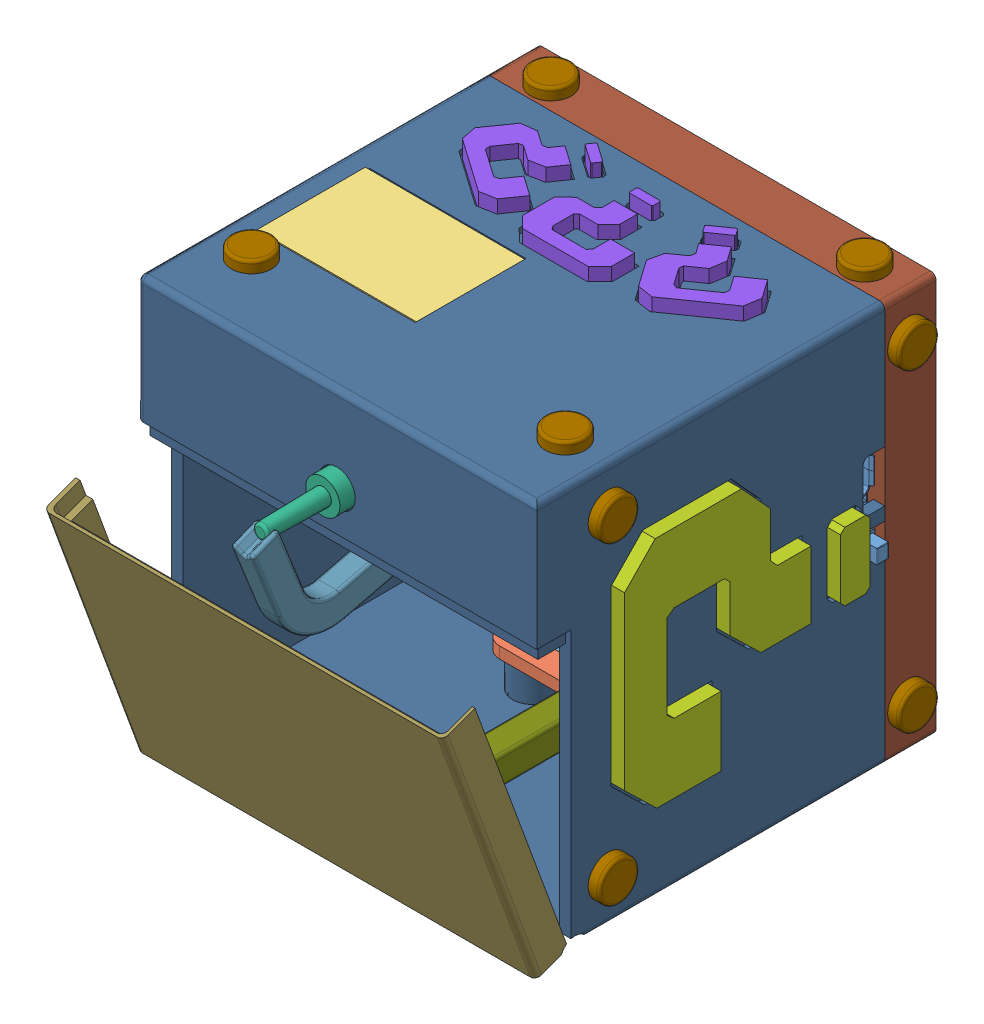
SolidWorks assembly 舔狗马里奥, configuration 默认. Lengths in mm.
Overall size (74.78 77.95 86.83).
34 component instances, 16 part files, 58 mates.
Components (placement in the parent):
- PCBA-1: PCBA [默认] at origin size (51.47 38.47 13.02)
- MP3模块-1: MP3模块 [默认] at (25.9874 -44.631 -27.0444) x (1 0 0) z (0 -1 0) size (40 32.5 9.5)
- OLED模块-1: OLED模块 [默认] at (-29.2626 11.569 29.8364) x (-1 0 0) z (0 1 0) size (28.5 28 22)
- 电池-1: 电池 [默认] at (-22.5126 -20.181 -82.6) x (0 0 -1) z (1 0 0) size (35.65 51.27 10)
- MG90S舵机-1: MG90S舵机 [默认] at (45.3874 0.569 27.75) x (0 0 1) z (0 -1 0) size (32.5 30.4 12.5)
- MG90S舵机-2: MG90S舵机 [默认] at (35.9874 -6.431 26.15) x (0 0 1) z (1 0 0) size (32.5 30.4 12.5)
- 开关-1: 开关 [默认] at (12.9874 0.569 47.9) x (-1 0 0) z (0 1 0) size (13 33 10)
- 马里奥问号-1: 马里奥问号 [默认] at (-21.0126 -25.4863 24.1423) x (0 1 0) z (0 0 1) size (41.06 3 43.04)
- 马里奥问号-2: 马里奥问号 [默认] at (18.3797 -53.431 24.146) x (-1 0 0) z (0 0 1) size (41.06 3 43.04)
- 马里奥问号-3: 马里奥问号 [默认] at (46.9874 -13.3946 24.3671) x (0 -1 0) z (0 0 1) size (41.06 3 43.04)
- 马里奥小问号-1: 马里奥小问号 [默认] at (-113.1118 14.569 -50.476) size (51.04 3 19.45)
- 马里奥键帽-1: 马里奥键帽 [默认] at (-21.0126 8.069 49.9) x (0 0.999538 0.03038) z (0 -0.03038 0.999538) size (7 3 7)
- 马里奥键帽-5: 马里奥键帽 [默认] at (-14.5126 -53.431 49.9) x (-0.990543 0 0.137199) z (0.137199 0 0.990543) size (7 3 7)
- 马里奥键帽-9: 马里奥键帽 [默认] at (46.9874 -46.931 49.9) x (0 -0.948117 -0.317921) z (0 -0.317921 0.948117) size (7 3 7)
- 马里奥键帽-13: 马里奥键帽 [默认] at (40.4874 14.569 49.9) x (0.738275 0 -0.6745) z (0.6745 0 0.738275) size (7 3 7)
- 马里奥盒子主体-1: 马里奥盒子主体 [默认] at (12.9874 -19.431 62.4) x (-1 0 0) z (0 -1 0) size (70 61 73.8)
- 马里奥盒子底座-1: 马里奥盒子底座 [默认] at (12.9874 -19.431 1.4) x (0 -1 0) z (1 0 0) size (70 9 70)
- 马里奥盖子-1: 马里奥盖子 [默认] at (12.9874 -33.6294 68.9166) x (1 0 0) z (0 -0.938921 -0.344132) size (70 11 51.55)
- 电池盖板-1: 电池盖板 [默认] at (-9.0126 -19.431 14.4) x (0 1 0) z (0 0 -1) size (60 2 36)
- 无聊杆-2: 无聊杆 [默认] at (14.9874 -3.8018 31.9291) x (0 -0.971273 -0.237969) z (-1 0 0) size (21.41 47.55 4)
- 马里奥键帽-3: 马里奥键帽 [默认] at (-21.0126 -46.931 49.9) x (0 0.999538 0.03038) z (0 -0.03038 0.999538) size (7 3 7)
- 马里奥键帽-7: 马里奥键帽 [默认] at (40.4874 -53.431 49.9) x (-0.990543 0 0.137199) z (0.137199 0 0.990543) size (7 3 7)
- 马里奥键帽-10: 马里奥键帽 [默认] at (46.9874 -46.931 -2.6) x (0 -0.948117 -0.317921) z (0 -0.317921 0.948117) size (7 3 7)
- 马里奥键帽-11: 马里奥键帽 [默认] at (46.9874 8.069 49.9) x (0 -0.948117 -0.317921) z (0 -0.317921 0.948117) size (7 3 7)
- 马里奥键帽-12: 马里奥键帽 [默认] at (46.9874 8.069 -2.6) x (0 -0.948117 -0.317921) z (0 -0.317921 0.948117) size (7 3 7)
- 马里奥键帽-14: 马里奥键帽 [默认] at (40.4874 14.569 -2.6) x (0.738275 0 -0.6745) z (0.6745 0 0.738275) size (7 3 7)
- 开盖杆-2: 开盖杆 [默认] at (30.9934 -38.831 31.1542) x (0.998791 0 0.049162) z (-0.049162 0 0.998791) size (18 2 5)
- 开盖杆B-1: 开盖杆B [默认] at (25.9995 -43.831 30.9084) x (0 0 1) z (-1 0 0) size (35.5 5.18 5)
- 马里奥键帽-17: 马里奥键帽 [默认] at (-21.0126 8.069 -2.6) x (0 0.999538 0.03038) z (0 -0.03038 0.999538) size (7 3 7)
- 马里奥键帽-18: 马里奥键帽 [默认] at (-21.0126 -46.931 -2.6) x (0 0.999538 0.03038) z (0 -0.03038 0.999538) size (7 3 7)
- 马里奥键帽-19: 马里奥键帽 [默认] at (-14.5126 -53.431 -2.6) x (-0.990543 0 0.137199) z (0.137199 0 0.990543) size (7 3 7)
- 马里奥键帽-20: 马里奥键帽 [默认] at (40.4874 -53.431 -2.6) x (-0.990543 0 0.137199) z (0.137199 0 0.990543) size (7 3 7)
- 马里奥键帽-21: 马里奥键帽 [默认] at (-14.5126 14.569 49.9) x (0.738275 0 -0.6745) z (0.6745 0 0.738275) size (7 3 7)
- 马里奥键帽-22: 马里奥键帽 [默认] at (-14.5126 14.569 -2.6) x (0.738275 0 -0.6745) z (0.6745 0 0.738275) size (7 3 7)
Mates (geometry in assembly coordinates):
- 重合1: coincident anti-aligned: plane of 马里奥盒子主体-1 through (12.9874 -19.431 1.4) normal (0 0 -1); plane of 马里奥盒子底座-1 through (12.9874 -19.431 1.4) normal (0 0 1)
- 重合2: coincident aligned: plane of 马里奥盒子主体-1 through (47.9874 15.569 1.4) normal (0 1 0); plane of 马里奥盒子底座-1 through (-22.0126 15.569 -7.6) normal (0 1 0)
- 重合3: coincident aligned: plane of 马里奥盒子主体-1 through (47.9874 15.569 1.4) normal (1 0 0); plane of 马里奥盒子底座-1 through (47.9874 15.569 -7.6) normal (1 0 0)
- 重合4: coincident anti-aligned: plane of 马里奥盒子底座-1 through (12.9874 -19.431 -5.6) normal (0 0 1); plane of PCBA-1 through (20.605 -35.4281 -5.6) normal (0 0 -1)
- 重合6: coincident anti-aligned: plane of PCBA-1 through (44.9874 -5 0) normal (1 0 0); plane of 马里奥盒子底座-1 through (44.9874 12.569 -98.1097) normal (-1 0 0)
- 宽度1: width aligned: plane of PCBA-1 through (50.769 -20.681 5.5079) normal (0 -1 0); plane of PCBA-1 through (50.769 -18.181 5.5079) normal (0 1 0); plane of 马里奥盒子底座-1 through (-22.0126 -54.431 -7.6) normal (0 -1 0); plane of 马里奥盒子底座-1 through (-22.0126 15.569 -7.6) normal (0 1 0)
- 重合8: coincident anti-aligned: plane of 电池-1 through (-22.5126 -20.181 -5.6) normal (0 0 -1); plane of 马里奥盒子底座-1 through (12.9874 -19.431 -5.6) normal (0 0 1)
- 宽度2: width anti-aligned: plane of 电池-1 through (-22.5126 6.319 -82.6) normal (0 1 0); plane of 马里奥盒子底座-1 through (-22.5126 -45.181 -82.6) normal (0 1 0); plane of 电池-1 through (44.9874 12.569 -98.1097) normal (0 -1 0); plane of 马里奥盒子底座-1 through (44.9874 -51.431 -98.1097) normal (0 1 0)
- 重合9: coincident aligned: plane of 电池-1 through (-19.0126 -20.181 -82.6) normal (1 0 0); plane of 马里奥盒子底座-1 through (-19.0126 12.569 -98.1097) normal (1 0 0)
- 重合12: coincident anti-aligned: plane of MP3模块-1 through (5.9874 -44.631 -5.6) normal (0 0 -1); plane of 马里奥盒子底座-1 through (12.9874 -19.431 -5.6) normal (0 0 1)
- 重合14: coincident anti-aligned: plane of OLED模块-1 through (-4.0126 13.569 35.2) normal (0 1 0); plane of 马里奥盒子主体-1 through (47.9874 13.569 1.4) normal (0 -1 0)
- 平行2: parallel aligned: plane of OLED模块-1 through (-16.7626 11.569 49.2) normal (0 0 1); plane of 马里奥盒子底座-1 through (12.9874 -19.431 -5.6) normal (0 0 1)
- 重合16: coincident anti-aligned: plane of MP3模块-1 through (7.2374 -52.431 10.65) normal (0 -1 0); plane of 马里奥盒子主体-1 through (47.9874 -52.431 1.4) normal (0 1 0)
- 距离1: distance = 5 mm aligned: plane of MP3模块-1 through (42.9874 -44.631 -2.6) normal (1 0 0); plane of 马里奥盒子底座-1 through (47.9874 15.569 -7.6) normal (1 0 0)
- 同心1: concentric anti-aligned: cylinder of 马里奥盒子主体-1 through (-16.0126 -19.431 32.4) axis (-1 0 0) radius 2.5; cylinder of 电池盖板-1 through (-7.0126 -19.431 32.4) axis (1 0 0) radius 1.7
- 相切4: tangent: plane of assembly; face of 电池-1; plane of 电池盖板-1 through (-9.0126 -19.431 14.4) normal (-1 0 0)
- 平行5: parallel aligned: plane of 马里奥盒子主体-1 through (47.9874 -54.431 56.4) normal (0 0 1); plane of 电池盖板-1 through (-7.0126 -44.431 29.9) normal (0 0 1)
- 平行6: parallel aligned: plane of MG90S舵机-1 through (29.3874 -5.681 39.25) normal (0 0 1); plane of 马里奥盒子主体-1 through (12.9874 -19.431 62.4) normal (0 0 1)
- 平行7: parallel aligned: plane of MG90S舵机-1 through (29.3874 -5.681 16.25) normal (0 -1 0); plane of 马里奥盒子主体-1 through (47.9874 -54.431 1.4) normal (0 -1 0)
- 同心2: concentric anti-aligned: cylinder of MG90S舵机-1 through (26.9874 0.569 41.5) axis (1 0 0) radius 1.5; cylinder of 马里奥盒子主体-1 through (47.9884 0.569 41.5) axis (-1 0 0) radius 1.25
- 重合20: coincident anti-aligned: plane of MG90S舵机-1 through (29.3874 0.569 27.75) normal (1 0 0); plane of 马里奥盒子主体-1 through (29.3874 -3.681 13.9) normal (-1 0 0)
- 宽度3: width anti-aligned: plane of 无聊杆-2 through (10.9874 -8.3743 65.2997) normal (-1 0 0); plane of 无聊杆-2 through (14.9874 -9.5007 32.0772) normal (1 0 0); plane of 马里奥盒子主体-1 through (47.9874 15.569 1.4) normal (1 0 0); plane of 马里奥盒子主体-1 through (-22.0126 15.569 1.4) normal (-1 0 0)
- 同心3: concentric aligned: circle of MG90S舵机-1; cylinder of 无聊杆-1 through (14.9874 0.569 33) axis (-1 0 0) radius 1.5
- 平行8: parallel anti-aligned: plane of 马里奥盒子主体-1 through (47.9874 15.569 1.4) normal (0 1 0); plane of 开关-1 through (19.4874 -4.431 55.9) normal (0 -1 0)
- 平行9: parallel aligned: plane of MG90S舵机-2 through (42.2374 -22.431 37.65) normal (0 0 1); plane of 马里奥盒子主体-1 through (12.9874 -19.431 62.4) normal (0 0 1)
- 平行10: parallel aligned: plane of MG90S舵机-2 through (42.2374 -22.431 14.65) normal (1 0 0); plane of 马里奥盒子底座-1 through (47.9874 15.569 -7.6) normal (1 0 0)
- 同心6: concentric anti-aligned: cylinder of MG90S舵机-2 through (35.9874 -24.831 39.9) axis (0 1 0) radius 1.5; cylinder of 马里奥盒子主体-1 through (35.9874 15.57 39.9) axis (0 -1 0) radius 1.25
- 重合26: coincident anti-aligned: plane of MG90S舵机-2 through (35.9874 -22.431 26.15) normal (0 1 0); plane of 马里奥盒子主体-1 through (31.7374 -22.431 39.4) normal (0 -1 0)
- 重合27: coincident anti-aligned: plane of 马里奥盒子主体-1 through (-21.0126 -19.431 62.4) normal (-1 0 0); plane of 马里奥问号-1 through (-21.0126 -25.4863 24.1423) normal (1 0 0)
- 宽度4: width anti-aligned: plane of 马里奥问号-1 through (-24.0126 -26.1306 22.0021) normal (0 -1 0); plane of 马里奥盒子主体-1 through (-24.0126 -14.3506 16.0741) normal (0 1 0); plane of 马里奥问号-1 through (-21.0126 -26.5306 21.8258) normal (0 1 0); plane of 马里奥盒子主体-1 through (-21.0126 -13.9506 15.6741) normal (0 -1 0)
- 宽度5: width anti-aligned: plane of 马里奥盒子主体-1 through (-21.0126 -14.6813 11.3457) normal (0 0 -1); plane of 马里奥问号-1 through (-21.0126 -14.6813 5.3457) normal (0 0 1); plane of 马里奥盒子主体-1 through (-24.0126 -14.8469 10.9457) normal (0 0 1); plane of 马里奥问号-1 through (-24.0126 -14.8469 5.7457) normal (0 0 -1)
- 重合28: coincident anti-aligned: plane of 马里奥盒子主体-1 through (12.9874 -53.431 62.4) normal (0 -1 0); plane of 马里奥问号-2 through (18.3797 -53.431 24.146) normal (0 1 0)
- 宽度6: width anti-aligned: plane of 马里奥问号-2 through (7.7403 -56.431 10.9495) normal (0 0 1); plane of 马里奥盒子主体-1 through (7.7403 -56.431 5.7495) normal (0 0 -1); plane of 马里奥问号-2 through (7.5747 -53.431 11.3495) normal (0 0 -1); plane of 马里奥盒子主体-1 through (7.5747 -53.431 5.3495) normal (0 0 1)
- 宽度7: width aligned: plane of 马里奥问号-2 through (18.9111 -56.431 10.1838) normal (1 0 0); plane of 马里奥盒子主体-1 through (6.9747 -56.431 10.1838) normal (-1 0 0); plane of 马里奥问号-2 through (6.5747 -53.431 10.3495) normal (1 0 0); plane of 马里奥盒子主体-1 through (19.3111 -53.431 10.3495) normal (-1 0 0)
- 重合29: coincident anti-aligned: plane of 马里奥盒子主体-1 through (46.9874 -19.431 62.4) normal (1 0 0); plane of 马里奥问号-3 through (46.9874 -13.3946 24.3671) normal (-1 0 0)
- 宽度8: width anti-aligned: plane of 马里奥问号-3 through (49.9874 -24.034 11.1706) normal (0 0 1); plane of 马里奥盒子主体-1 through (49.9874 -24.034 5.9706) normal (0 0 -1); plane of 马里奥问号-3 through (46.9874 -24.1997 11.5706) normal (0 0 -1); plane of 马里奥盒子主体-1 through (46.9874 -24.1997 5.5706) normal (0 0 1)
- 宽度9: width aligned: plane of 马里奥问号-3 through (49.9874 -24.7997 10.4049) normal (0 -1 0); plane of 马里奥盒子主体-1 through (49.9874 -12.8633 10.4049) normal (0 1 0); plane of 马里奥问号-3 through (46.9874 -12.4633 10.5706) normal (0 -1 0); plane of 马里奥盒子主体-1 through (46.9874 -25.1997 10.5706) normal (0 1 0)
- 重合31: coincident anti-aligned: plane of 马里奥盒子主体-1 through (12.9874 14.569 62.4) normal (0 1 0); plane of 马里奥小问号-1 through (-113.1118 14.569 -50.476) normal (0 -1 0)
- 宽度10: width anti-aligned: plane of 马里奥小问号-1 through (36.0745 17.569 10.0084) normal (0.819152 0 -0.573576); plane of 马里奥盒子主体-1 through (34.3509 17.569 14.9418) normal (-0.819152 0 0.573576); plane of 马里奥小问号-1 through (36.2249 14.569 9.5258) normal (-0.819152 0 0.573576); plane of 马里奥盒子主体-1 through (33.939 14.569 15.0509) normal (0.819152 0 -0.573576)
- 距离4: distance = 0.4 mm anti-aligned: plane of 马里奥小问号-1 through (32.6 17.569 12.4412) normal (-0.573576 0 -0.819152); plane of 马里奥盒子主体-1 through (32.0429 14.569 12.343) normal (0.573576 0 0.819152)
- 同心7: concentric anti-aligned: cylinder of 马里奥盒子主体-1 through (-21.0126 8.069 49.9) axis (-1 0 0) radius 2.5; cylinder of 马里奥键帽-1 through (-22.0126 8.069 49.9) axis (1 0 0) radius 2.3
- 重合32: coincident anti-aligned: plane of 马里奥盒子主体-1 through (-22.0126 15.569 1.4) normal (-1 0 0); plane of 马里奥键帽-1 through (-22.0126 8.069 49.9) normal (1 0 0)
- 同心8: concentric anti-aligned: cylinder of 马里奥盒子主体-1 through (-14.5126 -53.431 49.9) axis (0 -1 0) radius 2.5; cylinder of 马里奥键帽-5 through (-14.5126 -54.431 49.9) axis (0 1 0) radius 2.3
- 重合33: coincident anti-aligned: plane of 马里奥盒子主体-1 through (47.9874 -54.431 1.4) normal (0 -1 0); plane of 马里奥键帽-5 through (-14.5126 -54.431 49.9) normal (0 1 0)
- 同心9: concentric anti-aligned: cylinder of 马里奥盒子主体-1 through (46.9874 -46.931 49.9) axis (1 0 0) radius 2.5; cylinder of 马里奥键帽-9 through (47.9874 -46.931 49.9) axis (-1 0 0) radius 2.3
- 重合34: coincident anti-aligned: plane of 马里奥盒子主体-1 through (47.9874 15.569 1.4) normal (1 0 0); plane of 马里奥键帽-9 through (47.9874 -46.931 49.9) normal (-1 0 0)
- 同心10: concentric anti-aligned: cylinder of 马里奥盒子主体-1 through (40.4874 14.569 49.9) axis (0 1 0) radius 2.5; cylinder of 马里奥键帽-13 through (40.4874 15.569 49.9) axis (0 -1 0) radius 2.3
- 重合35: coincident anti-aligned: plane of 马里奥盒子主体-1 through (47.9874 15.569 1.4) normal (0 1 0); plane of 马里奥键帽-13 through (40.4874 15.569 49.9) normal (0 -1 0)
- 重合36: coincident aligned: plane of 马里奥盒子主体-1 through (-22.0126 15.569 1.4) normal (-1 0 0); plane of 马里奥盖子-1 through (-22.0126 -10.6773 75.309) normal (-1 0 0)
- 同心12: concentric aligned: cylinder of 马里奥盒子主体-1 through (-5.0126 -55.731 55.7) axis (-1 0 0) radius 1.25; cylinder of 马里奥盖子-1 through (47.9874 -55.731 55.7) axis (-1 0 0) radius 1.25
- 重合45: coincident anti-aligned: plane of MG90S舵机-2 through (35.9874 -36.831 31.4) normal (0 -1 0); plane of 开盖杆-2 through (38.0096 -36.831 30.9989) normal (0 1 0)
- 同心17: concentric anti-aligned: circle of MG90S舵机-2; cylinder of 开盖杆-2 through (35.9874 -38.831 31.4) axis (0 1 0) radius 1.5
- 同心18: concentric aligned: cylinder of 开盖杆-2 through (25.9995 -38.831 30.9084) axis (0 1 0) radius 1.65; cylinder of 开盖杆B-1 through (25.9995 -43.831 30.9084) axis (0 1 0) radius 1.4
- 重合46: coincident anti-aligned: plane of 开盖杆-2 through (38.0096 -38.831 30.9989) normal (0 -1 0); plane of 开盖杆B-1 through (25.9995 -38.831 30.9084) normal (0 1 0)
- 同心19: concentric anti-aligned: cylinder of 马里奥盖子-1 through (-22.0136 -41.8501 61.2696) axis (1 0 0) radius 1.5; cylinder of 开盖杆B-1 through (27.072 -41.331 59.1263) axis (-0.998652 0 -0.051914) radius 1.65
- 同心20: concentric aligned: cylinder of 开关-1 through (12.9874 0.569 64.9) axis (0 0 -1) radius 3; cylinder of 马里奥盒子主体-1 through (12.9874 0.569 62.401) axis (0 0 -1) radius 3.2
- 距离5: distance = 2.5 mm aligned: plane of 开关-1 through (12.9874 0.569 64.9) normal (0 0 1); plane of 马里奥盒子主体-1 through (12.9874 -19.431 62.4) normal (0 0 1)
- 平行12: parallel anti-aligned: plane of 马里奥盒子主体-1 through (-22.0126 15.569 1.4) normal (-1 0 0); plane of 开盖杆B-1 through (28.4995 -38.831 30.9084) normal (1 0 0)
